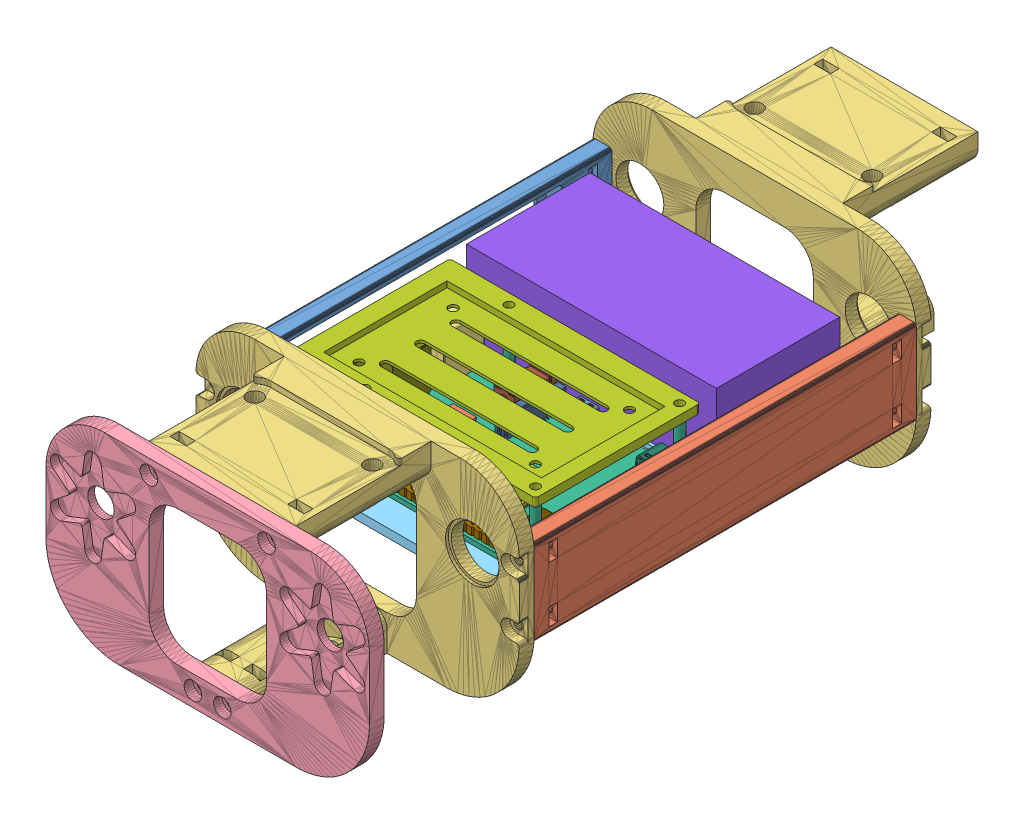
SolidWorks assembly torsol, configuration Default. Lengths in mm.
Overall size (110 70.14 237.21).
34 component instances, 26 part files, 36 mates.
Components (placement in the parent):
- R_side_plate_raspberry-1: R_side_plate_raspberry [Default] at (-145.3547 -0.5404 -42.0354) x (1 0 0) z (0 -1 0) size (6.5 130 29)
- non-mega_L_side_plate-2: non-mega_L_side_plate [Default] at (-41.8547 39.5958 -42.0354) x (-1 0 0) z (0 1 0) size (6.5 130 29)
- O_shoulder-1: O_shoulder [Default] at (-38.1905 81.6503 -93.0354) x (-1 0 0) z (0 -1 0) size (110 5.21 66) (hidden)
- I_shoulder_mg-1: I_shoulder_mg [Default] at (-38.6047 81.5958 -42.0354) x (-1 0 0) z (0 -1 0) size (110 51 70)
- I_shoulder_mg-2: I_shoulder_mg [Default] at (-148.6047 81.4596 87.9646) x (1 0 0) z (0 -1 0) size (110 51 70)
- O_shoulder-2: O_shoulder [Default] at (-148.6047 81.4596 138.9646) x (1 0 0) z (0 -1 0) size (110 5.21 66)
- plate_with_raspberry-1: plate_with_raspberry [Default] at (-77.9429 -68.9542 72.5105) x (1 0 0) z (0 1 0) size (107 125 22.11)
  - plate_raspberry-1: plate_raspberry [Default] at (-15.1617 3.5459 105.55) size (107 125 2.9)
  - Raspberry Pi 4 Model B-1: Raspberry Pi 4 Model B [Default] at (-14.6617 24.5459 110.6608) x (-1 0 0) z (0 1 0) size (88.99 19.9 58.4)
    - PCB, RPi4ModelB-1: PCB, RPi4ModelB [Default] at origin size (85 1.6 56)
    - Broadcom BCM2711B0 CPU, RPi4ModelB-1: Broadcom BCM2711B0 CPU, RPi4ModelB [Default] at (-13.25 0.8 -4.5) size (15 2.3 15)
    - 2.54 mm DUPONT MALE PIN HEADER, POE, 2X2, RPi4ModelB-1: 2.54 mm DUPONT MALE PIN HEADER, POE, 2X2, RPi4ModelB [Default] at (19 0.8 -18.5) size (5.08 11.3 5.08)
    - 2.54 mm DUPONT MALE PIN HEADER, IO, 2X20, RPi4ModelB-1: 2.54 mm DUPONT MALE PIN HEADER, IO, 2X20, RPi4ModelB [Default] at (-10 0.8 -24.5) size (50.8 11.3 5.08)
    - Camera Connector, RPi4ModelB-1: Camera Connector, RPi4ModelB [Default] at (4 0.8 16.5) x (0 0 -1) z (1 0 0) size (22.4 5.68 5.07)
    - Microphone Plug, RPi4ModelB-1: Microphone Plug, RPi4ModelB [Default] at (11.5 0.8 21.65) size (7.23 7.55 15)
    - Display Connector, RPi4ModelB-1: Display Connector, RPi4ModelB [Default] at (-38.5 0.8 0) x (0 0 1) z (-1 0 0) size (22.4 5.68 5.07)
    - Gigabit Ethernet Port, RPi4ModelB-1: Gigabit Ethernet Port, RPi4ModelB [Default] at (45.5 7.55 -17.75) x (0 0 -1) z (1 0 0) size (16.2 17.24 21.64)
    - Female Micro HDMI Connector, RPi4ModelB-2: Female Micro HDMI Connector, RPi4ModelB [Default] at (-3 0.8 27.3875) size (6.5 3.51 7.5)
    - Female Micro HDMI Connector, RPi4ModelB-3: Female Micro HDMI Connector, RPi4ModelB [Default] at (-16.5 0.8 27.3875) size (6.5 3.51 7.5)
    - Female USB Type C Connector, RPi4ModelB-1: Female USB Type C Connector, RPi4ModelB [Default] at (-31.3 0.8 26.5419) size (8.94 3.96 7.9)
    - 2X USB3.0 PORTS, RPi4ModelB-2: 2X USB3.0 PORTS, RPi4ModelB [Default] at (37.07 0.8 1) size (17.47 19.41 15.68)
    - 91D77 D9WHV 778K, 4 GB LPDDR4 SDRAM, RPi4ModelB-1: 91D77 D9WHV 778K, 4 GB LPDDR4 SDRAM, RPi4ModelB [Default] at (2.25 0.8 -4.5) size (10 0.8 14.5)
    - Cypress CYW43455 Wireless Module Cover, RPi4ModelB-1: Cypress CYW43455 Wireless Module Cover, RPi4ModelB [Default] at (-30.5 0.8 -14.5) size (11 1.6 13)
    - SD Card Slot, RPi4ModelB-1: SD Card Slot, RPi4ModelB [Default] at (-35.3 -0.8 0) x (0 0 -1) z (-1 0 0) size (11.95 1.45 11.4)
    - VIA VL805 PCIe USB 3.0 controller, RPi4ModelB-1: VIA VL805 PCIe USB 3.0 controller, RPi4ModelB [Default] at (17.5 0.8 4) size (8.8 0.8 8.8)
    - 2X USB2.0 PORTS, RPi4ModelB-1: 2X USB2.0 PORTS, RPi4ModelB [Default] at (37.065 0.65 19) size (17.87 19.16 15.33)
    - Broadcom BCM54213PE Gigabit Ethernet Transceiver, RPi4ModelB-1: Broadcom BCM54213PE Gigabit Ethernet Transceiver, RPi4ModelB [Default] at (16.5 0.8 -10) size (6.8 1 6.8)
    - MxL7704 Universal PMIC, RPi4ModelB-1: MxL7704 Universal PMIC, RPi4ModelB [Default] at (-32.5 0.8 16) size (5.4 0.8 5.4)
- copper_cylinder-1: copper_cylinder [Default] at (-111.6047 62.4966 72.4646) x (-0.975868 0 -0.218361) z (0 -1 0) size (3 3 20)
- copper_cylinder-2: copper_cylinder [Default] at (-53.6047 62.4966 72.4646) x (-0.932816 0 0.360352) z (0 -1 0) size (3 3 20)
- copper_cylinder-3: copper_cylinder [Default] at (-53.6047 62.4966 23.4646) x (-0.581089 0 -0.81384) z (0 -1 0) size (3 3 20)
- copper_cylinder-4: copper_cylinder [Default] at (-111.6047 62.4966 23.4646) x (-0.873325 0 -0.487138) z (0 -1 0) size (3 3 20)
- plate_top_raspberry-1: plate_top_raspberry [Default] at (-93.1414 65.3966 64.4169) x (1 0 0) z (0 -1 0) size (85.07 56 2.9)
- battery_4000mah_2s-1: battery_4000mah_2s [Default] at (-135.6047 66.4958 13.9646) x (1 0 0) z (0 -1 0) size (85 42 27)
Mates (geometry in assembly coordinates):
- Coincident9: coincident anti-aligned: plane of non-mega_L_side_plate-2 through (-41.8547 39.5958 -42.0354) normal (0 0 -1); plane of I_shoulder_mg-1 through (-38.6047 81.5958 -42.0354) normal (0 0 1)
- Parallel3: parallel anti-aligned: plane of R_side_plate_raspberry-1 through (-145.3547 -0.5404 -42.0354) normal (0 0 -1); plane of I_shoulder_mg-1 through (-38.6047 81.5958 -42.0354) normal (0 0 1)
- Parallel5: parallel aligned: plane of R_side_plate_raspberry-1 through (-145.3547 63.4596 -42.0354) normal (0 1 0); plane of I_shoulder_mg-1 through (-38.6047 81.5958 -42.0354) normal (0 1 0)
- Coincident20: coincident aligned: plane of R_side_plate_raspberry-1 through (-148.6047 -0.5404 -42.0354) normal (-1 0 0); plane of I_shoulder_mg-1 through (-148.6047 81.5958 -42.0354) normal (-1 0 0)
- Coincident22: coincident: point of R_side_plate_raspberry-1; plane of I_shoulder_mg-1 through (-66.0912 117.4171 -42.0354) normal (-0.60876 0.793355 0)
- Coincident23: coincident anti-aligned: plane of non-mega_L_side_plate-2 through (-41.8547 39.5958 87.9646) normal (0 0 1); plane of I_shoulder_mg-2 through (-148.6047 81.4596 87.9646) normal (0 0 -1)
- Coincident24: coincident aligned: plane of R_side_plate_raspberry-1 through (-148.6047 -0.5404 -42.0354) normal (-1 0 0); plane of I_shoulder_mg-2 through (-148.6047 81.4596 87.9646) normal (-1 0 0)
- Parallel7: parallel aligned: plane of R_side_plate_raspberry-1 through (-145.3547 63.4596 -42.0354) normal (0 1 0); plane of I_shoulder_mg-2 through (-148.6047 81.4596 87.9646) normal (0 1 0)
- Coincident26: coincident: plane of R_side_plate_raspberry-1 through (-137.9269 55.8817 -42.0354) normal (0.13052 0.991446 0); point of I_shoulder_mg-2
- Coincident27: coincident anti-aligned: plane of O_shoulder-1 through (-38.1905 81.6503 -93.0354) normal (0 0 1); plane of I_shoulder_mg-1 through (-38.6047 81.5958 -93.0354) normal (0 0 -1)
- Parallel8: parallel anti-aligned: plane of O_shoulder-1 through (-38.1905 13.6503 -93.0354) normal (0 -1 0); plane of I_shoulder_mg-1 through (-38.6047 79.5958 -42.0354) normal (0 1 0)
- Coincident29: coincident: point of O_shoulder-1; point of I_shoulder_mg-1
- Coincident30: coincident anti-aligned: plane of O_shoulder-2 through (-148.6047 81.4596 138.9646) normal (0 0 -1); plane of I_shoulder_mg-2 through (-148.6047 81.4596 138.9646) normal (0 0 1)
- Parallel9: parallel anti-aligned: plane of I_shoulder_mg-2 through (-148.6047 79.4596 87.9646) normal (0 1 0); plane of O_shoulder-2 through (-148.6047 13.4596 138.9646) normal (0 -1 0)
- Coincident32: coincident: point of I_shoulder_mg-2; point of O_shoulder-2
- Coincident33: coincident anti-aligned: plane of R_side_plate_raspberry-1 through (-145.3547 -0.5404 87.9646) normal (0 0 1); plane of I_shoulder_mg-2 through (-148.6047 81.4596 87.9646) normal (0 0 -1)
- Coincident34: coincident: point of non-mega_L_side_plate-2; point of I_shoulder_mg-1
- Parallel10: parallel aligned: plane of non-mega_L_side_plate-2 through (-41.8547 63.5958 -42.0354) normal (0 1 0); plane of I_shoulder_mg-1 through (-38.6047 81.5958 -42.0354) normal (0 1 0)
- Coincident37: coincident anti-aligned: plane of non-mega_L_side_plate-2 through (-39.6047 39.5958 -42.0354) normal (-1 0 0); plane of plate_with_raspberry-1/plate_raspberry-1 through (-39.6047 39.4958 68.9646) normal (1 0 0)
- Parallel11: parallel aligned: plane of I_shoulder_mg-1 through (-38.6047 81.5958 -47.0354) normal (0 0 -1); plane of plate_with_raspberry-1/plate_raspberry-1 through (-146.6047 39.4958 -26.0354) normal (0 0 -1)
- Coincident39: coincident anti-aligned: plane of non-mega_L_side_plate-2 through (-41.8547 36.5958 -42.0354) normal (0 1 0); plane of plate_with_raspberry-1/plate_raspberry-1 through (-93.1047 36.5958 68.9646) normal (0 -1 0)
- Concentric1: concentric anti-aligned: circle of plate_with_raspberry-1/Raspberry Pi 4 Model B-1/PCB, RPi4ModelB-1; circle of copper_cylinder-1
- Coincident40: coincident anti-aligned: plane of plate_with_raspberry-1/Raspberry Pi 4 Model B-1/PCB, RPi4ModelB-1 through (-111.6047 42.4966 72.4646) normal (0 1 0); circle of copper_cylinder-1
- Concentric3: concentric anti-aligned: circle of plate_with_raspberry-1/Raspberry Pi 4 Model B-1/PCB, RPi4ModelB-1; circle of copper_cylinder-2
- Coincident44: coincident anti-aligned: plane of plate_with_raspberry-1/Raspberry Pi 4 Model B-1/PCB, RPi4ModelB-1 through (-53.6047 42.4966 72.4646) normal (0 1 0); plane of copper_cylinder-2 through (-53.6047 42.4966 72.4646) normal (0 -1 0)
- Concentric4: concentric anti-aligned: circle of plate_with_raspberry-1/Raspberry Pi 4 Model B-1/PCB, RPi4ModelB-1; circle of copper_cylinder-3
- Coincident45: coincident anti-aligned: plane of plate_with_raspberry-1/Raspberry Pi 4 Model B-1/PCB, RPi4ModelB-1 through (-53.6047 42.4966 23.4646) normal (0 1 0); plane of copper_cylinder-3 through (-53.6047 42.4966 23.4646) normal (0 -1 0)
- Concentric5: concentric anti-aligned: circle of plate_with_raspberry-1/Raspberry Pi 4 Model B-1/PCB, RPi4ModelB-1; circle of copper_cylinder-4
- Coincident46: coincident anti-aligned: plane of plate_with_raspberry-1/Raspberry Pi 4 Model B-1/PCB, RPi4ModelB-1 through (-111.6047 42.4966 23.4646) normal (0 1 0); plane of copper_cylinder-4 through (-111.6047 42.4966 23.4646) normal (0 -1 0)
- Distance1: distance = 2 mm: line of plate_with_raspberry-1/plate_raspberry-1 through (-146.6047 39.4958 68.9646) axis (1 0 0); plane of non-mega_L_side_plate-2 through (-41.8547 39.5958 70.9646) normal (0 0 -1)
- Coincident52: coincident anti-aligned: plane of plate_with_raspberry-1/plate_raspberry-1 through (-93.1047 39.4958 68.9646) normal (0 1 0); plane of battery_4000mah_2s-1 through (-135.6047 39.4958 13.9646) normal (0 -1 0)
- Width1: width anti-aligned: plane of battery_4000mah_2s-1 through (-50.6047 39.4958 13.9646) normal (1 0 0); plane of battery_4000mah_2s-1 through (-135.6047 39.4958 13.9646) normal (-1 0 0); plane of plate_with_raspberry-1/plate_raspberry-1 through (-46.6047 39.4958 -14.0354) normal (-1 0 0); plane of plate_with_raspberry-1/plate_raspberry-1 through (-139.6047 39.4958 -14.0354) normal (1 0 0)
- Width2: width anti-aligned: plane of battery_4000mah_2s-1 through (-135.6047 39.4958 -28.0354) normal (0 0 -1); plane of battery_4000mah_2s-1 through (-135.6047 39.4958 13.9646) normal (0 0 1); plane of plate_with_raspberry-1/plate_raspberry-1 through (-132.1047 39.4958 -30.5354) normal (0 0 1); plane of plate_with_raspberry-1/plate_raspberry-1 through (-132.1047 39.4958 16.4646) normal (0 0 -1)
- Concentric14: concentric aligned: circle of copper_cylinder-2; circle of plate_top_raspberry-1
- Concentric15: concentric aligned: circle of copper_cylinder-4; circle of plate_top_raspberry-1
- Coincident53: coincident anti-aligned: plane of copper_cylinder-1 through (-111.6047 62.4966 72.4646) normal (0 1 0); plane of plate_top_raspberry-1 through (-93.1414 62.4966 64.4169) normal (0 -1 0)
